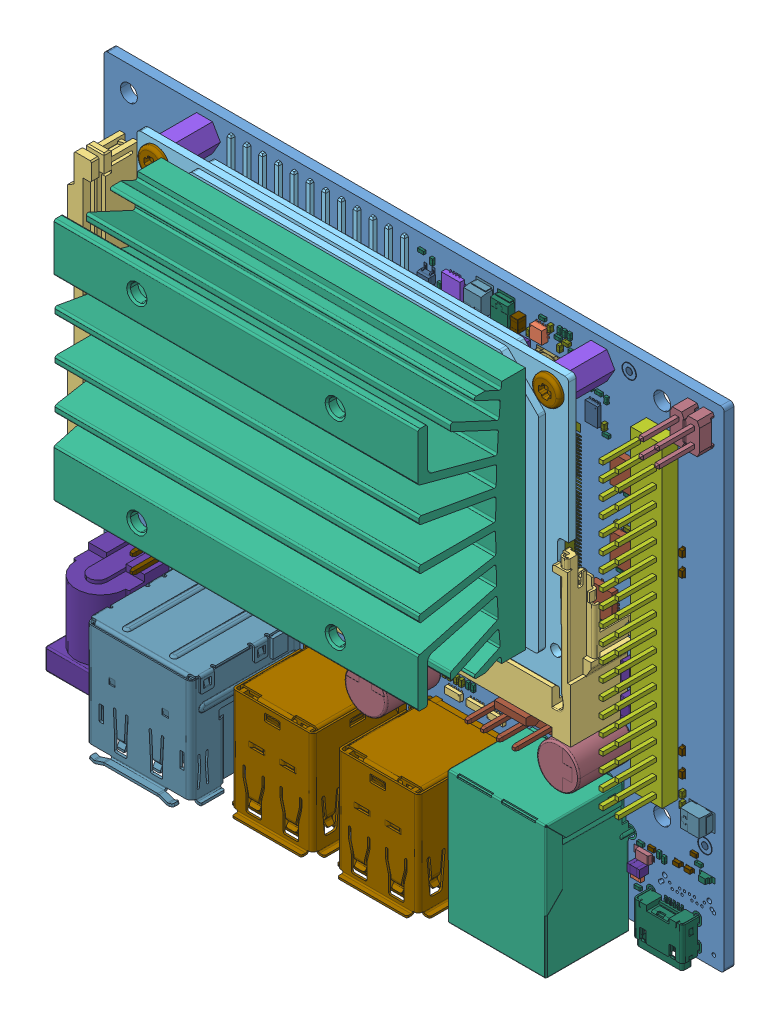
SolidWorks assembly Jetson_Nano_Dev_Kit_3D_b01, configuration Default. Lengths in mm. (continued)
Components (placement in the parent): (continued)
- Jetson_Nano_Dev_Kit_3D_b01(2)^Jetson_Nano_Dev_Kit_3D_b01-1: Jetson_Nano_Dev_Kit_3D_b01(2)^Jetson_Nano_Dev_Kit_3D_b01 [Default] at origin size (100 81.03 30.51) (virtual) (continued)
  - 642-13450_PORG_SYS_BOM^Jetson_Nano_Dev_Kit_3D_b01(2)_Jetson_Nano_Dev_Kit_3D_b01-1: 642-13450_PORG_SYS_BOM^Jetson_Nano_Dev_Kit_3D_b01(2)_Jetson_Nano_Dev_Kit_3D_b01 [Default] at origin size (100 81.03 23.18) (virtual) (continued)
    - 699-13449_PORG_DEV_KIT_PCB_ASSY^642-13450_PORG_SYS_BOM_Jetson_Nano_Dev_Kit_3D_b01(2)_Jetson_Nano_Dev_Kit_3D_b01-1: 699-13449_PORG_DEV_KIT_PCB_ASSY^642-13450_PORG_SYS_BOM_Jetson_Nano_Dev_Kit_3D_b01(2)_Jetson_Nano_Dev_Kit_3D_b01 [Default] at origin size (100 81.03 23.18) (virtual) (continued)
      - 600-13449_PORG_DEV_KIT_PCB_ASSY^699-13449_PORG_DEV_KIT_PCB_ASSY_642-13450_PORG_SYS_BOM_Jetson_Nano_Dev_Kit_3D_b01(2)_Jetson_Nano_Dev_Kit_3D_b01-1: 600-13449_PORG_DEV_KIT_PCB_ASSY^699-13449_PORG_DEV_KIT_PCB_ASSY_642-13450_PORG_SYS_BOM_Jetson_Nano_Dev_Kit_3D_b01(2)_Jetson_Nano_Dev_Kit_3D_b01 [Default] at origin size (100 81.03 23.18) (virtual) (continued)
        - 142-13449-1000-B01-SKU0000^600-13449_PORG_DEV_KIT_PCB_ASSY_699-13449_PORG_DEV_KIT_PCB_ASSY_642-13450_PORG_SYS_BOM_Jetson_Nano_Dev_Kit_3D_b01(2)_Jetson_Nano_Dev_Kit_3D_b01-1: 142-13449-1000-B01-SKU0000^600-13449_PORG_DEV_KIT_PCB_ASSY_699-13449_PORG_DEV_KIT_PCB_ASSY_642-13450_PORG_SYS_BOM_Jetson_Nano_Dev_Kit_3D_b01(2)_Jetson_Nano_Dev_Kit_3D_b01 [Default] at origin size (100 81.03 23.18) (virtual) (continued)
          - LOGO_SILK_HF_I0185X0120^142-13449-1000-B01-SKU0000_600-13449_PORG_DEV_KIT_PCB_ASSY_699-13449_PORG_DEV_KIT_PCB_ASSY_642-13450_PORG_SYS_BOM_Jetson_Nano_Dev_Kit_3D_b01(2)_Jetson_Nano_Dev_Kit_3D_b~-1: LOGO_SILK_HF_I0185X0120^142-13449-1000-B01-SKU0000_600-13449_PORG_DEV_KIT_PCB_ASSY_699-13449_PORG_DEV_KIT_PCB_ASSY_642-13450_PORG_SYS_BOM_Jetson_Nano_Dev_Kit_3D_b01(2)_Jetson_Nano_Dev_Kit_3D_b~ [Default] at (59.178 11.8 0) x (-1 0 0) z (0 0 -1) size (4.83 3.17 0.07) (virtual)
          - LOGO_SILK_BSMI_I0138H^142-13449-1000-B01-SKU0000_600-13449_PORG_DEV_KIT_PCB_ASSY_699-13449_PORG_DEV_KIT_PCB_ASSY_642-13450_PORG_SYS_BOM_Jetson_Nano_Dev_Kit_3D_b01(2)_Jetson_Nano_Dev_Kit_3D_b01-1: LOGO_SILK_BSMI_I0138H^142-13449-1000-B01-SKU0000_600-13449_PORG_DEV_KIT_PCB_ASSY_699-13449_PORG_DEV_KIT_PCB_ASSY_642-13450_PORG_SYS_BOM_Jetson_Nano_Dev_Kit_3D_b01(2)_Jetson_Nano_Dev_Kit_3D_b01 [Default] at (16.4 10.8 0) x (-1 0 0) z (0 0 -1) size (8.8 3.76 0.05) (virtual)
          - LOGO_SILK_RCM_040X030^142-13449-1000-B01-SKU0000_600-13449_PORG_DEV_KIT_PCB_ASSY_699-13449_PORG_DEV_KIT_PCB_ASSY_642-13450_PORG_SYS_BOM_Jetson_Nano_Dev_Kit_3D_b01(2)_Jetson_Nano_Dev_Kit_3D_b01-1: LOGO_SILK_RCM_040X030^142-13449-1000-B01-SKU0000_600-13449_PORG_DEV_KIT_PCB_ASSY_699-13449_PORG_DEV_KIT_PCB_ASSY_642-13450_PORG_SYS_BOM_Jetson_Nano_Dev_Kit_3D_b01(2)_Jetson_Nano_Dev_Kit_3D_b01 [Default] at (17.1 4.9 0) x (-1 0 0) z (0 0 -1) size (4.05 3 0.05) (virtual)
          - LOGO_SILK_VCCI_I0300X0225^142-13449-1000-B01-SKU0000_600-13449_PORG_DEV_KIT_PCB_ASSY_699-13449_PORG_DEV_KIT_PCB_ASSY_642-13450_PORG_SYS_BOM_Jetson_Nano_Dev_Kit_3D_b01(2)_Jetson_Nano_Dev_Kit_3D~-1: LOGO_SILK_VCCI_I0300X0225^142-13449-1000-B01-SKU0000_600-13449_PORG_DEV_KIT_PCB_ASSY_699-13449_PORG_DEV_KIT_PCB_ASSY_642-13450_PORG_SYS_BOM_Jetson_Nano_Dev_Kit_3D_b01(2)_Jetson_Nano_Dev_Kit_3D~ [Default] at (56.95 18.6 0) x (-1 0 0) z (0 0 -1) size (8.32 6.14 0.05) (virtual)
          - LOGO_SILK_WEEE_0485X0683^142-13449-1000-B01-SKU0000_600-13449_PORG_DEV_KIT_PCB_ASSY_699-13449_PORG_DEV_KIT_PCB_ASSY_642-13450_PORG_SYS_BOM_Jetson_Nano_Dev_Kit_3D_b01(2)_Jetson_Nano_Dev_Kit_3D_~-1: LOGO_SILK_WEEE_0485X0683^142-13449-1000-B01-SKU0000_600-13449_PORG_DEV_KIT_PCB_ASSY_699-13449_PORG_DEV_KIT_PCB_ASSY_642-13450_PORG_SYS_BOM_Jetson_Nano_Dev_Kit_3D_b01(2)_Jetson_Nano_Dev_Kit_3D_~ [Default] at (12.2 4.9 0) x (-1 0 0) z (0 0 -1) size (4.85 6.82 0.05) (virtual)
          - LOGO_SILK_ROHS_I0300X0153^142-13449-1000-B01-SKU0000_600-13449_PORG_DEV_KIT_PCB_ASSY_699-13449_PORG_DEV_KIT_PCB_ASSY_642-13450_PORG_SYS_BOM_Jetson_Nano_Dev_Kit_3D_b01(2)_Jetson_Nano_Dev_Kit_3D~-1: LOGO_SILK_ROHS_I0300X0153^142-13449-1000-B01-SKU0000_600-13449_PORG_DEV_KIT_PCB_ASSY_699-13449_PORG_DEV_KIT_PCB_ASSY_642-13450_PORG_SYS_BOM_Jetson_Nano_Dev_Kit_3D_b01(2)_Jetson_Nano_Dev_Kit_3D~ [Default] at (28.7 8.4 0) x (-1 0 0) z (0 0 -1) size (7.55 3.9 0.05) (virtual)
          - LOGO_SILK_ROHS_D050_CHINA^142-13449-1000-B01-SKU0000_600-13449_PORG_DEV_KIT_PCB_ASSY_699-13449_PORG_DEV_KIT_PCB_ASSY_642-13450_PORG_SYS_BOM_Jetson_Nano_Dev_Kit_3D_b01(2)_Jetson_Nano_Dev_Kit_3D~-1: LOGO_SILK_ROHS_D050_CHINA^142-13449-1000-B01-SKU0000_600-13449_PORG_DEV_KIT_PCB_ASSY_699-13449_PORG_DEV_KIT_PCB_ASSY_642-13450_PORG_SYS_BOM_Jetson_Nano_Dev_Kit_3D_b01(2)_Jetson_Nano_Dev_Kit_3D~ [Default] at (31.3 4.8 0) x (-1 0 0) z (0 0 -1) size (5.62 4.99 0.05) (virtual)
          - LOGO_SILK_NVIDIA_I0600X0330^142-13449-1000-B01-SKU0000_600-13449_PORG_DEV_KIT_PCB_ASSY_699-13449_PORG_DEV_KIT_PCB_ASSY_642-13450_PORG_SYS_BOM_Jetson_Nano_Dev_Kit_3D_b01(2)_Jetson_Nano_Dev_Kit_~-1: LOGO_SILK_NVIDIA_I0600X0330^142-13449-1000-B01-SKU0000_600-13449_PORG_DEV_KIT_PCB_ASSY_699-13449_PORG_DEV_KIT_PCB_ASSY_642-13450_PORG_SYS_BOM_Jetson_Nano_Dev_Kit_3D_b01(2)_Jetson_Nano_Dev_Kit_~ [Default] at (56.35 35.7 0) x (-1 0 0) z (0 0 -1) size (10.56 7.92 0.05) (virtual)
          - FID_40_80SM^142-13449-1000-B01-SKU0000_600-13449_PORG_DEV_KIT_PCB_ASSY_699-13449_PORG_DEV_KIT_PCB_ASSY_642-13450_PORG_SYS_BOM_Jetson_Nano_Dev_Kit_3D_b01(2)_Jetson_Nano_Dev_Kit_3D_b01-1: FID_40_80SM^142-13449-1000-B01-SKU0000_600-13449_PORG_DEV_KIT_PCB_ASSY_699-13449_PORG_DEV_KIT_PCB_ASSY_642-13450_PORG_SYS_BOM_Jetson_Nano_Dev_Kit_3D_b01(2)_Jetson_Nano_Dev_Kit_3D_b01 [Default] at (-0.15 -13.7 0) x (-1 0 0) z (0 0 -1) size (2.29 2.29 0.05) (virtual)
          - FID_40_80SM^142-13449-1000-B01-SKU0000_600-13449_PORG_DEV_KIT_PCB_ASSY_699-13449_PORG_DEV_KIT_PCB_ASSY_642-13450_PORG_SYS_BOM_Jetson_Nano_Dev_Kit_3D_b01(2)_Jetson_Nano_Dev_Kit_3D_b01-2: FID_40_80SM^142-13449-1000-B01-SKU0000_600-13449_PORG_DEV_KIT_PCB_ASSY_699-13449_PORG_DEV_KIT_PCB_ASSY_642-13450_PORG_SYS_BOM_Jetson_Nano_Dev_Kit_3D_b01(2)_Jetson_Nano_Dev_Kit_3D_b01 [Default] at (80.7 59.5 0) x (-1 0 0) z (0 0 -1) size (2.29 2.29 0.05) (virtual)
          - FID_40_80SM^142-13449-1000-B01-SKU0000_600-13449_PORG_DEV_KIT_PCB_ASSY_699-13449_PORG_DEV_KIT_PCB_ASSY_642-13450_PORG_SYS_BOM_Jetson_Nano_Dev_Kit_3D_b01(2)_Jetson_Nano_Dev_Kit_3D_b01-3: FID_40_80SM^142-13449-1000-B01-SKU0000_600-13449_PORG_DEV_KIT_PCB_ASSY_699-13449_PORG_DEV_KIT_PCB_ASSY_642-13450_PORG_SYS_BOM_Jetson_Nano_Dev_Kit_3D_b01(2)_Jetson_Nano_Dev_Kit_3D_b01 [Default] at (11.1 22.5 0) x (-1 0 0) z (0 0 -1) size (2.29 2.29 0.05) (virtual)
          - FID_40_80SM^142-13449-1000-B01-SKU0000_600-13449_PORG_DEV_KIT_PCB_ASSY_699-13449_PORG_DEV_KIT_PCB_ASSY_642-13450_PORG_SYS_BOM_Jetson_Nano_Dev_Kit_3D_b01(2)_Jetson_Nano_Dev_Kit_3D_b01-4: FID_40_80SM^142-13449-1000-B01-SKU0000_600-13449_PORG_DEV_KIT_PCB_ASSY_699-13449_PORG_DEV_KIT_PCB_ASSY_642-13450_PORG_SYS_BOM_Jetson_Nano_Dev_Kit_3D_b01(2)_Jetson_Nano_Dev_Kit_3D_b01 [Default] at (92.916 -0.657 1.57) size (2.29 2.29 0.05) (virtual)
          - FID_40_80SM^142-13449-1000-B01-SKU0000_600-13449_PORG_DEV_KIT_PCB_ASSY_699-13449_PORG_DEV_KIT_PCB_ASSY_642-13450_PORG_SYS_BOM_Jetson_Nano_Dev_Kit_3D_b01(2)_Jetson_Nano_Dev_Kit_3D_b01-5: FID_40_80SM^142-13449-1000-B01-SKU0000_600-13449_PORG_DEV_KIT_PCB_ASSY_699-13449_PORG_DEV_KIT_PCB_ASSY_642-13450_PORG_SYS_BOM_Jetson_Nano_Dev_Kit_3D_b01(2)_Jetson_Nano_Dev_Kit_3D_b01 [Default] at (4 52.9 1.57) size (2.29 2.29 0.05) (virtual)
          - FID_40_80SM^142-13449-1000-B01-SKU0000_600-13449_PORG_DEV_KIT_PCB_ASSY_699-13449_PORG_DEV_KIT_PCB_ASSY_642-13450_PORG_SYS_BOM_Jetson_Nano_Dev_Kit_3D_b01(2)_Jetson_Nano_Dev_Kit_3D_b01-6: FID_40_80SM^142-13449-1000-B01-SKU0000_600-13449_PORG_DEV_KIT_PCB_ASSY_699-13449_PORG_DEV_KIT_PCB_ASSY_642-13450_PORG_SYS_BOM_Jetson_Nano_Dev_Kit_3D_b01(2)_Jetson_Nano_Dev_Kit_3D_b01 [Default] at (80.7 59.5 1.57) size (2.29 2.29 0.05) (virtual)
          - 115-2177-000_2^142-13449-1000-B01-SKU0000_600-13449_PORG_DEV_KIT_PCB_ASSY_699-13449_PORG_DEV_KIT_PCB_ASSY_642-13450_PORG_SYS_BOM_Jetson_Nano_Dev_Kit_3D_b01(2)_Jetson_Nano_Dev_Kit_3D_b01-1: 115-2177-000_2^142-13449-1000-B01-SKU0000_600-13449_PORG_DEV_KIT_PCB_ASSY_699-13449_PORG_DEV_KIT_PCB_ASSY_642-13450_PORG_SYS_BOM_Jetson_Nano_Dev_Kit_3D_b01(2)_Jetson_Nano_Dev_Kit_3D_b01 [Default] at (41.5 46.3 1.57) size (1.8 1.71 0.4) (virtual)
          - 090-0378-000_1^142-13449-1000-B01-SKU0000_600-13449_PORG_DEV_KIT_PCB_ASSY_699-13449_PORG_DEV_KIT_PCB_ASSY_642-13450_PORG_SYS_BOM_Jetson_Nano_Dev_Kit_3D_b01(2)_Jetson_Nano_Dev_Kit_3D_b01-1: 090-0378-000_1^142-13449-1000-B01-SKU0000_600-13449_PORG_DEV_KIT_PCB_ASSY_699-13449_PORG_DEV_KIT_PCB_ASSY_642-13450_PORG_SYS_BOM_Jetson_Nano_Dev_Kit_3D_b01(2)_Jetson_Nano_Dev_Kit_3D_b01 [Default] at (6.85 -2.95 1.57) x (-1 0 0) z (0 0 1) size (3.3 1.3 0.73) (virtual)
          - 090-0233-000_1^142-13449-1000-B01-SKU0000_600-13449_PORG_DEV_KIT_PCB_ASSY_699-13449_PORG_DEV_KIT_PCB_ASSY_642-13450_PORG_SYS_BOM_Jetson_Nano_Dev_Kit_3D_b01(2)_Jetson_Nano_Dev_Kit_3D_b01-1: 090-0233-000_1^142-13449-1000-B01-SKU0000_600-13449_PORG_DEV_KIT_PCB_ASSY_699-13449_PORG_DEV_KIT_PCB_ASSY_642-13450_PORG_SYS_BOM_Jetson_Nano_Dev_Kit_3D_b01(2)_Jetson_Nano_Dev_Kit_3D_b01 [Default] at (83.5 -6.6 1.57) size (3.3 1.3 0.73) (virtual)
          - 064-0374-000_2^142-13449-1000-B01-SKU0000_600-13449_PORG_DEV_KIT_PCB_ASSY_699-13449_PORG_DEV_KIT_PCB_ASSY_642-13450_PORG_SYS_BOM_Jetson_Nano_Dev_Kit_3D_b01(2)_Jetson_Nano_Dev_Kit_3D_b01-1: 064-0374-000_2^142-13449-1000-B01-SKU0000_600-13449_PORG_DEV_KIT_PCB_ASSY_699-13449_PORG_DEV_KIT_PCB_ASSY_642-13450_PORG_SYS_BOM_Jetson_Nano_Dev_Kit_3D_b01(2)_Jetson_Nano_Dev_Kit_3D_b01 [Default] at (19.75 -9.65 1.57) size (18.1 18.55 21.85) (virtual)
          - 092-0073-000_1^142-13449-1000-B01-SKU0000_600-13449_PORG_DEV_KIT_PCB_ASSY_699-13449_PORG_DEV_KIT_PCB_ASSY_642-13450_PORG_SYS_BOM_Jetson_Nano_Dev_Kit_3D_b01(2)_Jetson_Nano_Dev_Kit_3D_b01-1: 092-0073-000_1^142-13449-1000-B01-SKU0000_600-13449_PORG_DEV_KIT_PCB_ASSY_699-13449_PORG_DEV_KIT_PCB_ASSY_642-13450_PORG_SYS_BOM_Jetson_Nano_Dev_Kit_3D_b01(2)_Jetson_Nano_Dev_Kit_3D_b01 [Default] at (93.35 -4.75 1.57) x (-1 0 0) z (0 0 1) size (2.46 0.81 0.9) (virtual)
          - IND_SMD_0402_H060^142-13449-1000-B01-SKU0000_600-13449_PORG_DEV_KIT_PCB_ASSY_699-13449_PORG_DEV_KIT_PCB_ASSY_642-13450_PORG_SYS_BOM_Jetson_Nano_Dev_Kit_3D_b01(2)_Jetson_Nano_Dev_Kit_3D_b01-1: IND_SMD_0402_H060^142-13449-1000-B01-SKU0000_600-13449_PORG_DEV_KIT_PCB_ASSY_699-13449_PORG_DEV_KIT_PCB_ASSY_642-13450_PORG_SYS_BOM_Jetson_Nano_Dev_Kit_3D_b01(2)_Jetson_Nano_Dev_Kit_3D_b01 [Default] at (11.65 37.2 1.57) x (0 -1 0) z (0 0 1) size (1 0.5 0.6) (virtual)
          - 1206_H190^142-13449-1000-B01-SKU0000_600-13449_PORG_DEV_KIT_PCB_ASSY_699-13449_PORG_DEV_KIT_PCB_ASSY_642-13450_PORG_SYS_BOM_Jetson_Nano_Dev_Kit_3D_b01(2)_Jetson_Nano_Dev_Kit_3D_b01-1: 1206_H190^142-13449-1000-B01-SKU0000_600-13449_PORG_DEV_KIT_PCB_ASSY_699-13449_PORG_DEV_KIT_PCB_ASSY_642-13450_PORG_SYS_BOM_Jetson_Nano_Dev_Kit_3D_b01(2)_Jetson_Nano_Dev_Kit_3D_b01 [Default] at (82 18.8 1.57) x (0 1 0) z (0 0 1) size (3.2 1.6 1.9) (virtual)
          - 1206_H190^142-13449-1000-B01-SKU0000_600-13449_PORG_DEV_KIT_PCB_ASSY_699-13449_PORG_DEV_KIT_PCB_ASSY_642-13450_PORG_SYS_BOM_Jetson_Nano_Dev_Kit_3D_b01(2)_Jetson_Nano_Dev_Kit_3D_b01-2: 1206_H190^142-13449-1000-B01-SKU0000_600-13449_PORG_DEV_KIT_PCB_ASSY_699-13449_PORG_DEV_KIT_PCB_ASSY_642-13450_PORG_SYS_BOM_Jetson_Nano_Dev_Kit_3D_b01(2)_Jetson_Nano_Dev_Kit_3D_b01 [Default] at (81.95 13.9 1.57) x (0 -1 0) z (0 0 1) size (3.2 1.6 1.9) (virtual)
          - 300-0868-000_3^142-13449-1000-B01-SKU0000_600-13449_PORG_DEV_KIT_PCB_ASSY_699-13449_PORG_DEV_KIT_PCB_ASSY_642-13450_PORG_SYS_BOM_Jetson_Nano_Dev_Kit_3D_b01(2)_Jetson_Nano_Dev_Kit_3D_b01-1: 300-0868-000_3^142-13449-1000-B01-SKU0000_600-13449_PORG_DEV_KIT_PCB_ASSY_699-13449_PORG_DEV_KIT_PCB_ASSY_642-13450_PORG_SYS_BOM_Jetson_Nano_Dev_Kit_3D_b01(2)_Jetson_Nano_Dev_Kit_3D_b01 [Default] at (45.25 48.45 1.57) size (1 0.6 0.4) (virtual)
          - 300-0868-000_3^142-13449-1000-B01-SKU0000_600-13449_PORG_DEV_KIT_PCB_ASSY_699-13449_PORG_DEV_KIT_PCB_ASSY_642-13450_PORG_SYS_BOM_Jetson_Nano_Dev_Kit_3D_b01(2)_Jetson_Nano_Dev_Kit_3D_b01-2: 300-0868-000_3^142-13449-1000-B01-SKU0000_600-13449_PORG_DEV_KIT_PCB_ASSY_699-13449_PORG_DEV_KIT_PCB_ASSY_642-13450_PORG_SYS_BOM_Jetson_Nano_Dev_Kit_3D_b01(2)_Jetson_Nano_Dev_Kit_3D_b01 [Default] at (73.85 3.9 1.57) x (-1 0 0) z (0 0 1) size (1 0.6 0.4) (virtual)
          - 300-0868-000_3^142-13449-1000-B01-SKU0000_600-13449_PORG_DEV_KIT_PCB_ASSY_699-13449_PORG_DEV_KIT_PCB_ASSY_642-13450_PORG_SYS_BOM_Jetson_Nano_Dev_Kit_3D_b01(2)_Jetson_Nano_Dev_Kit_3D_b01-3: 300-0868-000_3^142-13449-1000-B01-SKU0000_600-13449_PORG_DEV_KIT_PCB_ASSY_699-13449_PORG_DEV_KIT_PCB_ASSY_642-13450_PORG_SYS_BOM_Jetson_Nano_Dev_Kit_3D_b01(2)_Jetson_Nano_Dev_Kit_3D_b01 [Default] at (15.75 51.55 1.57) x (0 -1 0) z (0 0 1) size (1 0.6 0.4) (virtual)
          - 300-0868-000_3^142-13449-1000-B01-SKU0000_600-13449_PORG_DEV_KIT_PCB_ASSY_699-13449_PORG_DEV_KIT_PCB_ASSY_642-13450_PORG_SYS_BOM_Jetson_Nano_Dev_Kit_3D_b01(2)_Jetson_Nano_Dev_Kit_3D_b01-4: 300-0868-000_3^142-13449-1000-B01-SKU0000_600-13449_PORG_DEV_KIT_PCB_ASSY_699-13449_PORG_DEV_KIT_PCB_ASSY_642-13450_PORG_SYS_BOM_Jetson_Nano_Dev_Kit_3D_b01(2)_Jetson_Nano_Dev_Kit_3D_b01 [Default] at (11.5 34.8 1.57) x (0 1 0) z (0 0 1) size (1 0.6 0.4) (virtual)
          - 300-0868-000_3^142-13449-1000-B01-SKU0000_600-13449_PORG_DEV_KIT_PCB_ASSY_699-13449_PORG_DEV_KIT_PCB_ASSY_642-13450_PORG_SYS_BOM_Jetson_Nano_Dev_Kit_3D_b01(2)_Jetson_Nano_Dev_Kit_3D_b01-5: 300-0868-000_3^142-13449-1000-B01-SKU0000_600-13449_PORG_DEV_KIT_PCB_ASSY_699-13449_PORG_DEV_KIT_PCB_ASSY_642-13450_PORG_SYS_BOM_Jetson_Nano_Dev_Kit_3D_b01(2)_Jetson_Nano_Dev_Kit_3D_b01 [Default] at (91.45 -2.45 1.57) x (-1 0 0) z (0 0 1) size (1 0.6 0.4) (virtual)
          - 300-0868-000_3^142-13449-1000-B01-SKU0000_600-13449_PORG_DEV_KIT_PCB_ASSY_699-13449_PORG_DEV_KIT_PCB_ASSY_642-13450_PORG_SYS_BOM_Jetson_Nano_Dev_Kit_3D_b01(2)_Jetson_Nano_Dev_Kit_3D_b01-6: 300-0868-000_3^142-13449-1000-B01-SKU0000_600-13449_PORG_DEV_KIT_PCB_ASSY_699-13449_PORG_DEV_KIT_PCB_ASSY_642-13450_PORG_SYS_BOM_Jetson_Nano_Dev_Kit_3D_b01(2)_Jetson_Nano_Dev_Kit_3D_b01 [Default] at (84.6 -5.1 1.57) size (1 0.6 0.4) (virtual)
          - 300-0868-000_3^142-13449-1000-B01-SKU0000_600-13449_PORG_DEV_KIT_PCB_ASSY_699-13449_PORG_DEV_KIT_PCB_ASSY_642-13450_PORG_SYS_BOM_Jetson_Nano_Dev_Kit_3D_b01(2)_Jetson_Nano_Dev_Kit_3D_b01-7: 300-0868-000_3^142-13449-1000-B01-SKU0000_600-13449_PORG_DEV_KIT_PCB_ASSY_699-13449_PORG_DEV_KIT_PCB_ASSY_642-13450_PORG_SYS_BOM_Jetson_Nano_Dev_Kit_3D_b01(2)_Jetson_Nano_Dev_Kit_3D_b01 [Default] at (11.9 32.55 1.57) x (-1 0 0) z (0 0 1) size (1 0.6 0.4) (virtual)
          - 300-0868-000_3^142-13449-1000-B01-SKU0000_600-13449_PORG_DEV_KIT_PCB_ASSY_699-13449_PORG_DEV_KIT_PCB_ASSY_642-13450_PORG_SYS_BOM_Jetson_Nano_Dev_Kit_3D_b01(2)_Jetson_Nano_Dev_Kit_3D_b01-8: 300-0868-000_3^142-13449-1000-B01-SKU0000_600-13449_PORG_DEV_KIT_PCB_ASSY_699-13449_PORG_DEV_KIT_PCB_ASSY_642-13450_PORG_SYS_BOM_Jetson_Nano_Dev_Kit_3D_b01(2)_Jetson_Nano_Dev_Kit_3D_b01 [Default] at (62.85 28.15 1.57) x (-1 0 0) z (0 0 1) size (1 0.6 0.4) (virtual)
          - 300-0868-000_3^142-13449-1000-B01-SKU0000_600-13449_PORG_DEV_KIT_PCB_ASSY_699-13449_PORG_DEV_KIT_PCB_ASSY_642-13450_PORG_SYS_BOM_Jetson_Nano_Dev_Kit_3D_b01(2)_Jetson_Nano_Dev_Kit_3D_b01-9: 300-0868-000_3^142-13449-1000-B01-SKU0000_600-13449_PORG_DEV_KIT_PCB_ASSY_699-13449_PORG_DEV_KIT_PCB_ASSY_642-13450_PORG_SYS_BOM_Jetson_Nano_Dev_Kit_3D_b01(2)_Jetson_Nano_Dev_Kit_3D_b01 [Default] at (62.4 30.55 1.57) x (-1 0 0) z (0 0 1) size (1 0.6 0.4) (virtual)
          - 300-0868-000_3^142-13449-1000-B01-SKU0000_600-13449_PORG_DEV_KIT_PCB_ASSY_699-13449_PORG_DEV_KIT_PCB_ASSY_642-13450_PORG_SYS_BOM_Jetson_Nano_Dev_Kit_3D_b01(2)_Jetson_Nano_Dev_Kit_3D_b01-10: 300-0868-000_3^142-13449-1000-B01-SKU0000_600-13449_PORG_DEV_KIT_PCB_ASSY_699-13449_PORG_DEV_KIT_PCB_ASSY_642-13450_PORG_SYS_BOM_Jetson_Nano_Dev_Kit_3D_b01(2)_Jetson_Nano_Dev_Kit_3D_b01 [Default] at (11.4 41.6 1.57) x (-1 0 0) z (0 0 1) size (1 0.6 0.4) (virtual)
          - 300-0868-000_3^142-13449-1000-B01-SKU0000_600-13449_PORG_DEV_KIT_PCB_ASSY_699-13449_PORG_DEV_KIT_PCB_ASSY_642-13450_PORG_SYS_BOM_Jetson_Nano_Dev_Kit_3D_b01(2)_Jetson_Nano_Dev_Kit_3D_b01-11: 300-0868-000_3^142-13449-1000-B01-SKU0000_600-13449_PORG_DEV_KIT_PCB_ASSY_699-13449_PORG_DEV_KIT_PCB_ASSY_642-13450_PORG_SYS_BOM_Jetson_Nano_Dev_Kit_3D_b01(2)_Jetson_Nano_Dev_Kit_3D_b01 [Default] at (11.8 6.1 1.57) x (0 1 0) z (0 0 1) size (1 0.6 0.4) (virtual)
          - 300-0869-000_3^142-13449-1000-B01-SKU0000_600-13449_PORG_DEV_KIT_PCB_ASSY_699-13449_PORG_DEV_KIT_PCB_ASSY_642-13450_PORG_SYS_BOM_Jetson_Nano_Dev_Kit_3D_b01(2)_Jetson_Nano_Dev_Kit_3D_b01-1: 300-0869-000_3^142-13449-1000-B01-SKU0000_600-13449_PORG_DEV_KIT_PCB_ASSY_699-13449_PORG_DEV_KIT_PCB_ASSY_642-13450_PORG_SYS_BOM_Jetson_Nano_Dev_Kit_3D_b01(2)_Jetson_Nano_Dev_Kit_3D_b01 [Default] at (9.65 8.1 1.57) x (0 -1 0) z (0 0 1) size (1 0.6 0.53) (virtual)
          - 115-1968-000_2^142-13449-1000-B01-SKU0000_600-13449_PORG_DEV_KIT_PCB_ASSY_699-13449_PORG_DEV_KIT_PCB_ASSY_642-13450_PORG_SYS_BOM_Jetson_Nano_Dev_Kit_3D_b01(2)_Jetson_Nano_Dev_Kit_3D_b01-1: 115-1968-000_2^142-13449-1000-B01-SKU0000_600-13449_PORG_DEV_KIT_PCB_ASSY_699-13449_PORG_DEV_KIT_PCB_ASSY_642-13450_PORG_SYS_BOM_Jetson_Nano_Dev_Kit_3D_b01(2)_Jetson_Nano_Dev_Kit_3D_b01 [Default] at (61.25 6.85 1.57) x (0 -1 0) z (0 0 1) size (2 2.69 1.2) (virtual)
          - 115-1566-000_1^142-13449-1000-B01-SKU0000_600-13449_PORG_DEV_KIT_PCB_ASSY_699-13449_PORG_DEV_KIT_PCB_ASSY_642-13450_PORG_SYS_BOM_Jetson_Nano_Dev_Kit_3D_b01(2)_Jetson_Nano_Dev_Kit_3D_b01-1: 115-1566-000_1^142-13449-1000-B01-SKU0000_600-13449_PORG_DEV_KIT_PCB_ASSY_699-13449_PORG_DEV_KIT_PCB_ASSY_642-13450_PORG_SYS_BOM_Jetson_Nano_Dev_Kit_3D_b01(2)_Jetson_Nano_Dev_Kit_3D_b01 [Default] at (48.25 50.3 1.57) x (-1 0 0) z (0 0 1) size (2 2.69 1.1) (virtual)
          - 300-0402-000_1^142-13449-1000-B01-SKU0000_600-13449_PORG_DEV_KIT_PCB_ASSY_699-13449_PORG_DEV_KIT_PCB_ASSY_642-13450_PORG_SYS_BOM_Jetson_Nano_Dev_Kit_3D_b01(2)_Jetson_Nano_Dev_Kit_3D_b01-1: 300-0402-000_1^142-13449-1000-B01-SKU0000_600-13449_PORG_DEV_KIT_PCB_ASSY_699-13449_PORG_DEV_KIT_PCB_ASSY_642-13450_PORG_SYS_BOM_Jetson_Nano_Dev_Kit_3D_b01(2)_Jetson_Nano_Dev_Kit_3D_b01 [Default] at (13.65 44.4 1.57) x (0 1 0) z (0 0 1) size (2 2.69 1.1) (virtual)
          - 300-0560-000_1^142-13449-1000-B01-SKU0000_600-13449_PORG_DEV_KIT_PCB_ASSY_699-13449_PORG_DEV_KIT_PCB_ASSY_642-13450_PORG_SYS_BOM_Jetson_Nano_Dev_Kit_3D_b01(2)_Jetson_Nano_Dev_Kit_3D_b01-1: 300-0560-000_1^142-13449-1000-B01-SKU0000_600-13449_PORG_DEV_KIT_PCB_ASSY_699-13449_PORG_DEV_KIT_PCB_ASSY_642-13450_PORG_SYS_BOM_Jetson_Nano_Dev_Kit_3D_b01(2)_Jetson_Nano_Dev_Kit_3D_b01 [Default] at (31.2 45.2 1.57) x (-1 0 0) z (0 0 1) size (2 2.69 1.1) (virtual)
          - 064-0404-000_1^142-13449-1000-B01-SKU0000_600-13449_PORG_DEV_KIT_PCB_ASSY_699-13449_PORG_DEV_KIT_PCB_ASSY_642-13450_PORG_SYS_BOM_Jetson_Nano_Dev_Kit_3D_b01(2)_Jetson_Nano_Dev_Kit_3D_b01-1: 064-0404-000_1^142-13449-1000-B01-SKU0000_600-13449_PORG_DEV_KIT_PCB_ASSY_699-13449_PORG_DEV_KIT_PCB_ASSY_642-13450_PORG_SYS_BOM_Jetson_Nano_Dev_Kit_3D_b01(2)_Jetson_Nano_Dev_Kit_3D_b01 [Default] at (72.95 -7.825 1.57) size (17.8 21.6 17.45) (virtual)
          - 074-0221-000_3^142-13449-1000-B01-SKU0000_600-13449_PORG_DEV_KIT_PCB_ASSY_699-13449_PORG_DEV_KIT_PCB_ASSY_642-13450_PORG_SYS_BOM_Jetson_Nano_Dev_Kit_3D_b01(2)_Jetson_Nano_Dev_Kit_3D_b01-1: 074-0221-000_3^142-13449-1000-B01-SKU0000_600-13449_PORG_DEV_KIT_PCB_ASSY_699-13449_PORG_DEV_KIT_PCB_ASSY_642-13450_PORG_SYS_BOM_Jetson_Nano_Dev_Kit_3D_b01(2)_Jetson_Nano_Dev_Kit_3D_b01 [Default] at (86 29 1.57) x (0 1 0) z (0 0 1) size (50.8 5.08 11.6) (virtual)
          - 2016MM_H100^142-13449-1000-B01-SKU0000_600-13449_PORG_DEV_KIT_PCB_ASSY_699-13449_PORG_DEV_KIT_PCB_ASSY_642-13450_PORG_SYS_BOM_Jetson_Nano_Dev_Kit_3D_b01(2)_Jetson_Nano_Dev_Kit_3D_b01-1: 2016MM_H100^142-13449-1000-B01-SKU0000_600-13449_PORG_DEV_KIT_PCB_ASSY_699-13449_PORG_DEV_KIT_PCB_ASSY_642-13450_PORG_SYS_BOM_Jetson_Nano_Dev_Kit_3D_b01(2)_Jetson_Nano_Dev_Kit_3D_b01 [Default] at (23 43.25 1.57) x (0 1 0) z (0 0 1) size (2 1.6 1) (virtual)
          - 065-0656-000_2^142-13449-1000-B01-SKU0000_600-13449_PORG_DEV_KIT_PCB_ASSY_699-13449_PORG_DEV_KIT_PCB_ASSY_642-13450_PORG_SYS_BOM_Jetson_Nano_Dev_Kit_3D_b01(2)_Jetson_Nano_Dev_Kit_3D_b01-1: 065-0656-000_2^142-13449-1000-B01-SKU0000_600-13449_PORG_DEV_KIT_PCB_ASSY_699-13449_PORG_DEV_KIT_PCB_ASSY_642-13450_PORG_SYS_BOM_Jetson_Nano_Dev_Kit_3D_b01(2)_Jetson_Nano_Dev_Kit_3D_b01 [Default] at (55.6 -10.04 1.57) x (-1 0 0) z (0 0 1) size (16.19 17.45 19.64) (virtual)
          - 065-0656-000_2^142-13449-1000-B01-SKU0000_600-13449_PORG_DEV_KIT_PCB_ASSY_699-13449_PORG_DEV_KIT_PCB_ASSY_642-13450_PORG_SYS_BOM_Jetson_Nano_Dev_Kit_3D_b01(2)_Jetson_Nano_Dev_Kit_3D_b01-2: 065-0656-000_2^142-13449-1000-B01-SKU0000_600-13449_PORG_DEV_KIT_PCB_ASSY_699-13449_PORG_DEV_KIT_PCB_ASSY_642-13450_PORG_SYS_BOM_Jetson_Nano_Dev_Kit_3D_b01(2)_Jetson_Nano_Dev_Kit_3D_b01 [Default] at (38.6 -10.04 1.57) x (-1 0 0) z (0 0 1) size (16.19 17.45 19.64) (virtual)
          - LOGO_SILK_180_I560^142-13449-1000-B01-SKU0000_600-13449_PORG_DEV_KIT_PCB_ASSY_699-13449_PORG_DEV_KIT_PCB_ASSY_642-13450_PORG_SYS_BOM_Jetson_Nano_Dev_Kit_3D_b01(2)_Jetson_Nano_Dev_Kit_3D_b01-1: LOGO_SILK_180_I560^142-13449-1000-B01-SKU0000_600-13449_PORG_DEV_KIT_PCB_ASSY_699-13449_PORG_DEV_KIT_PCB_ASSY_642-13450_PORG_SYS_BOM_Jetson_Nano_Dev_Kit_3D_b01(2)_Jetson_Nano_Dev_Kit_3D_b01 [Default] at (61.45 24.95 0) x (-1 0 0) z (0 0 -1) size (14.3 1.27 0.05) (virtual)
          - 115-1921-000_3^142-13449-1000-B01-SKU0000_600-13449_PORG_DEV_KIT_PCB_ASSY_699-13449_PORG_DEV_KIT_PCB_ASSY_642-13450_PORG_SYS_BOM_Jetson_Nano_Dev_Kit_3D_b01(2)_Jetson_Nano_Dev_Kit_3D_b01-1: 115-1921-000_3^142-13449-1000-B01-SKU0000_600-13449_PORG_DEV_KIT_PCB_ASSY_699-13449_PORG_DEV_KIT_PCB_ASSY_642-13450_PORG_SYS_BOM_Jetson_Nano_Dev_Kit_3D_b01(2)_Jetson_Nano_Dev_Kit_3D_b01 [Default] at (80.45 45.52 1.57) x (0 -1 0) z (0 0 1) size (5 4 1) (virtual)
          - 115-1921-000_3^142-13449-1000-B01-SKU0000_600-13449_PORG_DEV_KIT_PCB_ASSY_699-13449_PORG_DEV_KIT_PCB_ASSY_642-13450_PORG_SYS_BOM_Jetson_Nano_Dev_Kit_3D_b01(2)_Jetson_Nano_Dev_Kit_3D_b01-2: 115-1921-000_3^142-13449-1000-B01-SKU0000_600-13449_PORG_DEV_KIT_PCB_ASSY_699-13449_PORG_DEV_KIT_PCB_ASSY_642-13450_PORG_SYS_BOM_Jetson_Nano_Dev_Kit_3D_b01(2)_Jetson_Nano_Dev_Kit_3D_b01 [Default] at (80.4 34.5 1.57) x (0 -1 0) z (0 0 1) size (5 4 1) (virtual)
          - 115-1921-000_3^142-13449-1000-B01-SKU0000_600-13449_PORG_DEV_KIT_PCB_ASSY_699-13449_PORG_DEV_KIT_PCB_ASSY_642-13450_PORG_SYS_BOM_Jetson_Nano_Dev_Kit_3D_b01(2)_Jetson_Nano_Dev_Kit_3D_b01-3: 115-1921-000_3^142-13449-1000-B01-SKU0000_600-13449_PORG_DEV_KIT_PCB_ASSY_699-13449_PORG_DEV_KIT_PCB_ASSY_642-13450_PORG_SYS_BOM_Jetson_Nano_Dev_Kit_3D_b01(2)_Jetson_Nano_Dev_Kit_3D_b01 [Default] at (77.2 25.9 1.57) x (0 -1 0) z (0 0 1) size (5 4 1) (virtual)
          - 085-0328-000_2^142-13449-1000-B01-SKU0000_600-13449_PORG_DEV_KIT_PCB_ASSY_699-13449_PORG_DEV_KIT_PCB_ASSY_642-13450_PORG_SYS_BOM_Jetson_Nano_Dev_Kit_3D_b01(2)_Jetson_Nano_Dev_Kit_3D_b01-1: 085-0328-000_2^142-13449-1000-B01-SKU0000_600-13449_PORG_DEV_KIT_PCB_ASSY_699-13449_PORG_DEV_KIT_PCB_ASSY_642-13450_PORG_SYS_BOM_Jetson_Nano_Dev_Kit_3D_b01(2)_Jetson_Nano_Dev_Kit_3D_b01 [Default] at (14.78 30.32 1.57) x (0 -1 0) z (0 0 1) size (3.81 2.5 0.6) (virtual)
          - 074-0216-000_2^142-13449-1000-B01-SKU0000_600-13449_PORG_DEV_KIT_PCB_ASSY_699-13449_PORG_DEV_KIT_PCB_ASSY_642-13450_PORG_SYS_BOM_Jetson_Nano_Dev_Kit_3D_b01(2)_Jetson_Nano_Dev_Kit_3D_b01-1: 074-0216-000_2^142-13449-1000-B01-SKU0000_600-13449_PORG_DEV_KIT_PCB_ASSY_699-13449_PORG_DEV_KIT_PCB_ASSY_642-13450_PORG_SYS_BOM_Jetson_Nano_Dev_Kit_3D_b01(2)_Jetson_Nano_Dev_Kit_3D_b01 [Default] at (92.14 58 1.57) x (-1 0 0) z (0 0 1) size (4.83 5 11.5) (virtual)
          - 032-0696-000_1^142-13449-1000-B01-SKU0000_600-13449_PORG_DEV_KIT_PCB_ASSY_699-13449_PORG_DEV_KIT_PCB_ASSY_642-13450_PORG_SYS_BOM_Jetson_Nano_Dev_Kit_3D_b01(2)_Jetson_Nano_Dev_Kit_3D_b01-1: 032-0696-000_1^142-13449-1000-B01-SKU0000_600-13449_PORG_DEV_KIT_PCB_ASSY_699-13449_PORG_DEV_KIT_PCB_ASSY_642-13450_PORG_SYS_BOM_Jetson_Nano_Dev_Kit_3D_b01(2)_Jetson_Nano_Dev_Kit_3D_b01 [Default] at (7.1 5.5 1.57) size (4.22 2.82 2) (virtual)
          - 032-0696-000_1^142-13449-1000-B01-SKU0000_600-13449_PORG_DEV_KIT_PCB_ASSY_699-13449_PORG_DEV_KIT_PCB_ASSY_642-13450_PORG_SYS_BOM_Jetson_Nano_Dev_Kit_3D_b01(2)_Jetson_Nano_Dev_Kit_3D_b01-2: 032-0696-000_1^142-13449-1000-B01-SKU0000_600-13449_PORG_DEV_KIT_PCB_ASSY_699-13449_PORG_DEV_KIT_PCB_ASSY_642-13450_PORG_SYS_BOM_Jetson_Nano_Dev_Kit_3D_b01(2)_Jetson_Nano_Dev_Kit_3D_b01 [Default] at (92.5 3.3 1.57) size (4.22 2.82 2) (virtual)
          - 032-0696-000_1^142-13449-1000-B01-SKU0000_600-13449_PORG_DEV_KIT_PCB_ASSY_699-13449_PORG_DEV_KIT_PCB_ASSY_642-13450_PORG_SYS_BOM_Jetson_Nano_Dev_Kit_3D_b01(2)_Jetson_Nano_Dev_Kit_3D_b01-3: 032-0696-000_1^142-13449-1000-B01-SKU0000_600-13449_PORG_DEV_KIT_PCB_ASSY_699-13449_PORG_DEV_KIT_PCB_ASSY_642-13450_PORG_SYS_BOM_Jetson_Nano_Dev_Kit_3D_b01(2)_Jetson_Nano_Dev_Kit_3D_b01 [Default] at (57.45 58.4 1.57) x (0 1 0) z (0 0 1) size (4.22 2.82 2) (virtual)
          - 041-0092-000_1^142-13449-1000-B01-SKU0000_600-13449_PORG_DEV_KIT_PCB_ASSY_699-13449_PORG_DEV_KIT_PCB_ASSY_642-13450_PORG_SYS_BOM_Jetson_Nano_Dev_Kit_3D_b01(2)_Jetson_Nano_Dev_Kit_3D_b01-1: 041-0092-000_1^142-13449-1000-B01-SKU0000_600-13449_PORG_DEV_KIT_PCB_ASSY_699-13449_PORG_DEV_KIT_PCB_ASSY_642-13450_PORG_SYS_BOM_Jetson_Nano_Dev_Kit_3D_b01(2)_Jetson_Nano_Dev_Kit_3D_b01 [Default] at (60.95 58.4 1.57) x (0 -1 0) z (0 0 1) size (4.22 2.82 1.2) (virtual)
          - 080-1243-000_3^142-13449-1000-B01-SKU0000_600-13449_PORG_DEV_KIT_PCB_ASSY_699-13449_PORG_DEV_KIT_PCB_ASSY_642-13450_PORG_SYS_BOM_Jetson_Nano_Dev_Kit_3D_b01(2)_Jetson_Nano_Dev_Kit_3D_b01-1: 080-1243-000_3^142-13449-1000-B01-SKU0000_600-13449_PORG_DEV_KIT_PCB_ASSY_699-13449_PORG_DEV_KIT_PCB_ASSY_642-13450_PORG_SYS_BOM_Jetson_Nano_Dev_Kit_3D_b01(2)_Jetson_Nano_Dev_Kit_3D_b01 [Default] at (68.4 37.3 1.57) x (0 -1 0) z (0 0 1) size (21.9 9.1 4.8) (virtual)
          - 0805_H150^142-13449-1000-B01-SKU0000_600-13449_PORG_DEV_KIT_PCB_ASSY_699-13449_PORG_DEV_KIT_PCB_ASSY_642-13450_PORG_SYS_BOM_Jetson_Nano_Dev_Kit_3D_b01(2)_Jetson_Nano_Dev_Kit_3D_b01-1: 0805_H150^142-13449-1000-B01-SKU0000_600-13449_PORG_DEV_KIT_PCB_ASSY_699-13449_PORG_DEV_KIT_PCB_ASSY_642-13450_PORG_SYS_BOM_Jetson_Nano_Dev_Kit_3D_b01(2)_Jetson_Nano_Dev_Kit_3D_b01 [Default] at (63.8 55.3 1.57) x (-1 0 0) z (0 0 1) size (2.01 1.25 1.5) (virtual)
          - 0805_H150^142-13449-1000-B01-SKU0000_600-13449_PORG_DEV_KIT_PCB_ASSY_699-13449_PORG_DEV_KIT_PCB_ASSY_642-13450_PORG_SYS_BOM_Jetson_Nano_Dev_Kit_3D_b01(2)_Jetson_Nano_Dev_Kit_3D_b01-2: 0805_H150^142-13449-1000-B01-SKU0000_600-13449_PORG_DEV_KIT_PCB_ASSY_699-13449_PORG_DEV_KIT_PCB_ASSY_642-13450_PORG_SYS_BOM_Jetson_Nano_Dev_Kit_3D_b01(2)_Jetson_Nano_Dev_Kit_3D_b01 [Default] at (63.8 53.5 1.57) x (-1 0 0) z (0 0 1) size (2.01 1.25 1.5) (virtual)
          - 0805_H140^142-13449-1000-B01-SKU0000_600-13449_PORG_DEV_KIT_PCB_ASSY_699-13449_PORG_DEV_KIT_PCB_ASSY_642-13450_PORG_SYS_BOM_Jetson_Nano_Dev_Kit_3D_b01(2)_Jetson_Nano_Dev_Kit_3D_b01-1: 0805_H140^142-13449-1000-B01-SKU0000_600-13449_PORG_DEV_KIT_PCB_ASSY_699-13449_PORG_DEV_KIT_PCB_ASSY_642-13450_PORG_SYS_BOM_Jetson_Nano_Dev_Kit_3D_b01(2)_Jetson_Nano_Dev_Kit_3D_b01 [Default] at (63.55 58.1 1.57) x (0 -1 0) z (0 0 1) size (2.01 1.25 1.4) (virtual)
          - 0805_H140^142-13449-1000-B01-SKU0000_600-13449_PORG_DEV_KIT_PCB_ASSY_699-13449_PORG_DEV_KIT_PCB_ASSY_642-13450_PORG_SYS_BOM_Jetson_Nano_Dev_Kit_3D_b01(2)_Jetson_Nano_Dev_Kit_3D_b01-2: 0805_H140^142-13449-1000-B01-SKU0000_600-13449_PORG_DEV_KIT_PCB_ASSY_699-13449_PORG_DEV_KIT_PCB_ASSY_642-13450_PORG_SYS_BOM_Jetson_Nano_Dev_Kit_3D_b01(2)_Jetson_Nano_Dev_Kit_3D_b01 [Default] at (58.4 54.65 1.57) size (2.01 1.25 1.4) (virtual)
          - 0805_H150^142-13449-1000-B01-SKU0000_600-13449_PORG_DEV_KIT_PCB_ASSY_699-13449_PORG_DEV_KIT_PCB_ASSY_642-13450_PORG_SYS_BOM_Jetson_Nano_Dev_Kit_3D_b01(2)_Jetson_Nano_Dev_Kit_3D_b01-3: 0805_H150^142-13449-1000-B01-SKU0000_600-13449_PORG_DEV_KIT_PCB_ASSY_699-13449_PORG_DEV_KIT_PCB_ASSY_642-13450_PORG_SYS_BOM_Jetson_Nano_Dev_Kit_3D_b01(2)_Jetson_Nano_Dev_Kit_3D_b01 [Default] at (63.8 51.75 1.57) x (-1 0 0) z (0 0 1) size (2.01 1.25 1.5) (virtual)
          - 0805_H150^142-13449-1000-B01-SKU0000_600-13449_PORG_DEV_KIT_PCB_ASSY_699-13449_PORG_DEV_KIT_PCB_ASSY_642-13450_PORG_SYS_BOM_Jetson_Nano_Dev_Kit_3D_b01(2)_Jetson_Nano_Dev_Kit_3D_b01-4: 0805_H150^142-13449-1000-B01-SKU0000_600-13449_PORG_DEV_KIT_PCB_ASSY_699-13449_PORG_DEV_KIT_PCB_ASSY_642-13450_PORG_SYS_BOM_Jetson_Nano_Dev_Kit_3D_b01(2)_Jetson_Nano_Dev_Kit_3D_b01 [Default] at (-0.95 5.45 1.57) x (-1 0 0) z (0 0 1) size (2.01 1.25 1.5) (virtual)
          - 0805_H150^142-13449-1000-B01-SKU0000_600-13449_PORG_DEV_KIT_PCB_ASSY_699-13449_PORG_DEV_KIT_PCB_ASSY_642-13450_PORG_SYS_BOM_Jetson_Nano_Dev_Kit_3D_b01(2)_Jetson_Nano_Dev_Kit_3D_b01-5: 0805_H150^142-13449-1000-B01-SKU0000_600-13449_PORG_DEV_KIT_PCB_ASSY_699-13449_PORG_DEV_KIT_PCB_ASSY_642-13450_PORG_SYS_BOM_Jetson_Nano_Dev_Kit_3D_b01(2)_Jetson_Nano_Dev_Kit_3D_b01 [Default] at (82.9 -8.4 1.57) x (-1 0 0) z (0 0 1) size (2.01 1.25 1.5) (virtual)
          - 0603_H100^142-13449-1000-B01-SKU0000_600-13449_PORG_DEV_KIT_PCB_ASSY_699-13449_PORG_DEV_KIT_PCB_ASSY_642-13450_PORG_SYS_BOM_Jetson_Nano_Dev_Kit_3D_b01(2)_Jetson_Nano_Dev_Kit_3D_b01-1: 0603_H100^142-13449-1000-B01-SKU0000_600-13449_PORG_DEV_KIT_PCB_ASSY_699-13449_PORG_DEV_KIT_PCB_ASSY_642-13450_PORG_SYS_BOM_Jetson_Nano_Dev_Kit_3D_b01(2)_Jetson_Nano_Dev_Kit_3D_b01 [Default] at (58.35 8.5 1.57) x (0 1 0) z (0 0 1) size (1.6 0.81 1) (virtual)
          - 0603_H100^142-13449-1000-B01-SKU0000_600-13449_PORG_DEV_KIT_PCB_ASSY_699-13449_PORG_DEV_KIT_PCB_ASSY_642-13450_PORG_SYS_BOM_Jetson_Nano_Dev_Kit_3D_b01(2)_Jetson_Nano_Dev_Kit_3D_b01-2: 0603_H100^142-13449-1000-B01-SKU0000_600-13449_PORG_DEV_KIT_PCB_ASSY_699-13449_PORG_DEV_KIT_PCB_ASSY_642-13450_PORG_SYS_BOM_Jetson_Nano_Dev_Kit_3D_b01(2)_Jetson_Nano_Dev_Kit_3D_b01 [Default] at (31.05 43.05 1.57) x (-1 0 0) z (0 0 1) size (1.6 0.81 1) (virtual)
          - 0603_H060^142-13449-1000-B01-SKU0000_600-13449_PORG_DEV_KIT_PCB_ASSY_699-13449_PORG_DEV_KIT_PCB_ASSY_642-13450_PORG_SYS_BOM_Jetson_Nano_Dev_Kit_3D_b01(2)_Jetson_Nano_Dev_Kit_3D_b01-1: 0603_H060^142-13449-1000-B01-SKU0000_600-13449_PORG_DEV_KIT_PCB_ASSY_699-13449_PORG_DEV_KIT_PCB_ASSY_642-13450_PORG_SYS_BOM_Jetson_Nano_Dev_Kit_3D_b01(2)_Jetson_Nano_Dev_Kit_3D_b01 [Default] at (63.25 -12 1.57) x (0 1 0) z (0 0 1) size (1.6 0.81 0.6) (virtual)
          - 0603_H060^142-13449-1000-B01-SKU0000_600-13449_PORG_DEV_KIT_PCB_ASSY_699-13449_PORG_DEV_KIT_PCB_ASSY_642-13450_PORG_SYS_BOM_Jetson_Nano_Dev_Kit_3D_b01(2)_Jetson_Nano_Dev_Kit_3D_b01-2: 0603_H060^142-13449-1000-B01-SKU0000_600-13449_PORG_DEV_KIT_PCB_ASSY_699-13449_PORG_DEV_KIT_PCB_ASSY_642-13450_PORG_SYS_BOM_Jetson_Nano_Dev_Kit_3D_b01(2)_Jetson_Nano_Dev_Kit_3D_b01 [Default] at (63.8 -0.7 1.57) x (0 -1 0) z (0 0 1) size (1.6 0.81 0.6) (virtual)
          - 0603_H060^142-13449-1000-B01-SKU0000_600-13449_PORG_DEV_KIT_PCB_ASSY_699-13449_PORG_DEV_KIT_PCB_ASSY_642-13450_PORG_SYS_BOM_Jetson_Nano_Dev_Kit_3D_b01(2)_Jetson_Nano_Dev_Kit_3D_b01-3: 0603_H060^142-13449-1000-B01-SKU0000_600-13449_PORG_DEV_KIT_PCB_ASSY_699-13449_PORG_DEV_KIT_PCB_ASSY_642-13450_PORG_SYS_BOM_Jetson_Nano_Dev_Kit_3D_b01(2)_Jetson_Nano_Dev_Kit_3D_b01 [Default] at (82.4 -10 1.57) x (-1 0 0) z (0 0 1) size (1.6 0.81 0.6) (virtual)
          - 0603_H100^142-13449-1000-B01-SKU0000_600-13449_PORG_DEV_KIT_PCB_ASSY_699-13449_PORG_DEV_KIT_PCB_ASSY_642-13450_PORG_SYS_BOM_Jetson_Nano_Dev_Kit_3D_b01(2)_Jetson_Nano_Dev_Kit_3D_b01-3: 0603_H100^142-13449-1000-B01-SKU0000_600-13449_PORG_DEV_KIT_PCB_ASSY_699-13449_PORG_DEV_KIT_PCB_ASSY_642-13450_PORG_SYS_BOM_Jetson_Nano_Dev_Kit_3D_b01(2)_Jetson_Nano_Dev_Kit_3D_b01 [Default] at (10.35 -9.5 1.57) x (0 -1 0) z (0 0 1) size (1.6 0.81 1) (virtual)
          - 0603_H100^142-13449-1000-B01-SKU0000_600-13449_PORG_DEV_KIT_PCB_ASSY_699-13449_PORG_DEV_KIT_PCB_ASSY_642-13450_PORG_SYS_BOM_Jetson_Nano_Dev_Kit_3D_b01(2)_Jetson_Nano_Dev_Kit_3D_b01-4: 0603_H100^142-13449-1000-B01-SKU0000_600-13449_PORG_DEV_KIT_PCB_ASSY_699-13449_PORG_DEV_KIT_PCB_ASSY_642-13450_PORG_SYS_BOM_Jetson_Nano_Dev_Kit_3D_b01(2)_Jetson_Nano_Dev_Kit_3D_b01 [Default] at (21.75 47.05 1.57) x (0 -1 0) z (0 0 1) size (1.6 0.81 1) (virtual)
          - 0603_H100^142-13449-1000-B01-SKU0000_600-13449_PORG_DEV_KIT_PCB_ASSY_699-13449_PORG_DEV_KIT_PCB_ASSY_642-13450_PORG_SYS_BOM_Jetson_Nano_Dev_Kit_3D_b01(2)_Jetson_Nano_Dev_Kit_3D_b01-5: 0603_H100^142-13449-1000-B01-SKU0000_600-13449_PORG_DEV_KIT_PCB_ASSY_699-13449_PORG_DEV_KIT_PCB_ASSY_642-13450_PORG_SYS_BOM_Jetson_Nano_Dev_Kit_3D_b01(2)_Jetson_Nano_Dev_Kit_3D_b01 [Default] at (35.15 43.15 1.57) x (0 1 0) z (0 0 1) size (1.6 0.81 1) (virtual)
          - 0603_H100^142-13449-1000-B01-SKU0000_600-13449_PORG_DEV_KIT_PCB_ASSY_699-13449_PORG_DEV_KIT_PCB_ASSY_642-13450_PORG_SYS_BOM_Jetson_Nano_Dev_Kit_3D_b01(2)_Jetson_Nano_Dev_Kit_3D_b01-6: 0603_H100^142-13449-1000-B01-SKU0000_600-13449_PORG_DEV_KIT_PCB_ASSY_699-13449_PORG_DEV_KIT_PCB_ASSY_642-13450_PORG_SYS_BOM_Jetson_Nano_Dev_Kit_3D_b01(2)_Jetson_Nano_Dev_Kit_3D_b01 [Default] at (60.2 49.2 1.57) x (-1 0 0) z (0 0 1) size (1.6 0.81 1) (virtual)
          - 0603_H100^142-13449-1000-B01-SKU0000_600-13449_PORG_DEV_KIT_PCB_ASSY_699-13449_PORG_DEV_KIT_PCB_ASSY_642-13450_PORG_SYS_BOM_Jetson_Nano_Dev_Kit_3D_b01(2)_Jetson_Nano_Dev_Kit_3D_b01-7: 0603_H100^142-13449-1000-B01-SKU0000_600-13449_PORG_DEV_KIT_PCB_ASSY_699-13449_PORG_DEV_KIT_PCB_ASSY_642-13450_PORG_SYS_BOM_Jetson_Nano_Dev_Kit_3D_b01(2)_Jetson_Nano_Dev_Kit_3D_b01 [Default] at (61.1 54.35 1.57) x (-1 0 0) z (0 0 1) size (1.6 0.81 1) (virtual)
          - 0603_H100^142-13449-1000-B01-SKU0000_600-13449_PORG_DEV_KIT_PCB_ASSY_699-13449_PORG_DEV_KIT_PCB_ASSY_642-13450_PORG_SYS_BOM_Jetson_Nano_Dev_Kit_3D_b01(2)_Jetson_Nano_Dev_Kit_3D_b01-8: 0603_H100^142-13449-1000-B01-SKU0000_600-13449_PORG_DEV_KIT_PCB_ASSY_699-13449_PORG_DEV_KIT_PCB_ASSY_642-13450_PORG_SYS_BOM_Jetson_Nano_Dev_Kit_3D_b01(2)_Jetson_Nano_Dev_Kit_3D_b01 [Default] at (26.95 43.65 1.57) x (0 -1 0) z (0 0 1) size (1.6 0.81 1) (virtual)
          - 0603_H100^142-13449-1000-B01-SKU0000_600-13449_PORG_DEV_KIT_PCB_ASSY_699-13449_PORG_DEV_KIT_PCB_ASSY_642-13450_PORG_SYS_BOM_Jetson_Nano_Dev_Kit_3D_b01(2)_Jetson_Nano_Dev_Kit_3D_b01-9: 0603_H100^142-13449-1000-B01-SKU0000_600-13449_PORG_DEV_KIT_PCB_ASSY_699-13449_PORG_DEV_KIT_PCB_ASSY_642-13450_PORG_SYS_BOM_Jetson_Nano_Dev_Kit_3D_b01(2)_Jetson_Nano_Dev_Kit_3D_b01 [Default] at (21.2 43.1 1.57) x (0 1 0) z (0 0 1) size (1.6 0.81 1) (virtual)
          - 0603_H100^142-13449-1000-B01-SKU0000_600-13449_PORG_DEV_KIT_PCB_ASSY_699-13449_PORG_DEV_KIT_PCB_ASSY_642-13450_PORG_SYS_BOM_Jetson_Nano_Dev_Kit_3D_b01(2)_Jetson_Nano_Dev_Kit_3D_b01-10: 0603_H100^142-13449-1000-B01-SKU0000_600-13449_PORG_DEV_KIT_PCB_ASSY_699-13449_PORG_DEV_KIT_PCB_ASSY_642-13450_PORG_SYS_BOM_Jetson_Nano_Dev_Kit_3D_b01(2)_Jetson_Nano_Dev_Kit_3D_b01 [Default] at (24.7 42.25 1.57) x (0 1 0) z (0 0 1) size (1.6 0.81 1) (virtual)
          - 0603_H100^142-13449-1000-B01-SKU0000_600-13449_PORG_DEV_KIT_PCB_ASSY_699-13449_PORG_DEV_KIT_PCB_ASSY_642-13450_PORG_SYS_BOM_Jetson_Nano_Dev_Kit_3D_b01(2)_Jetson_Nano_Dev_Kit_3D_b01-11: 0603_H100^142-13449-1000-B01-SKU0000_600-13449_PORG_DEV_KIT_PCB_ASSY_699-13449_PORG_DEV_KIT_PCB_ASSY_642-13450_PORG_SYS_BOM_Jetson_Nano_Dev_Kit_3D_b01(2)_Jetson_Nano_Dev_Kit_3D_b01 [Default] at (19.4 43.1 1.57) x (0 1 0) z (0 0 1) size (1.6 0.81 1) (virtual)
          - 0603_H100^142-13449-1000-B01-SKU0000_600-13449_PORG_DEV_KIT_PCB_ASSY_699-13449_PORG_DEV_KIT_PCB_ASSY_642-13450_PORG_SYS_BOM_Jetson_Nano_Dev_Kit_3D_b01(2)_Jetson_Nano_Dev_Kit_3D_b01-12: 0603_H100^142-13449-1000-B01-SKU0000_600-13449_PORG_DEV_KIT_PCB_ASSY_699-13449_PORG_DEV_KIT_PCB_ASSY_642-13450_PORG_SYS_BOM_Jetson_Nano_Dev_Kit_3D_b01(2)_Jetson_Nano_Dev_Kit_3D_b01 [Default] at (65.85 49.2 1.57) size (1.6 0.81 1) (virtual)
